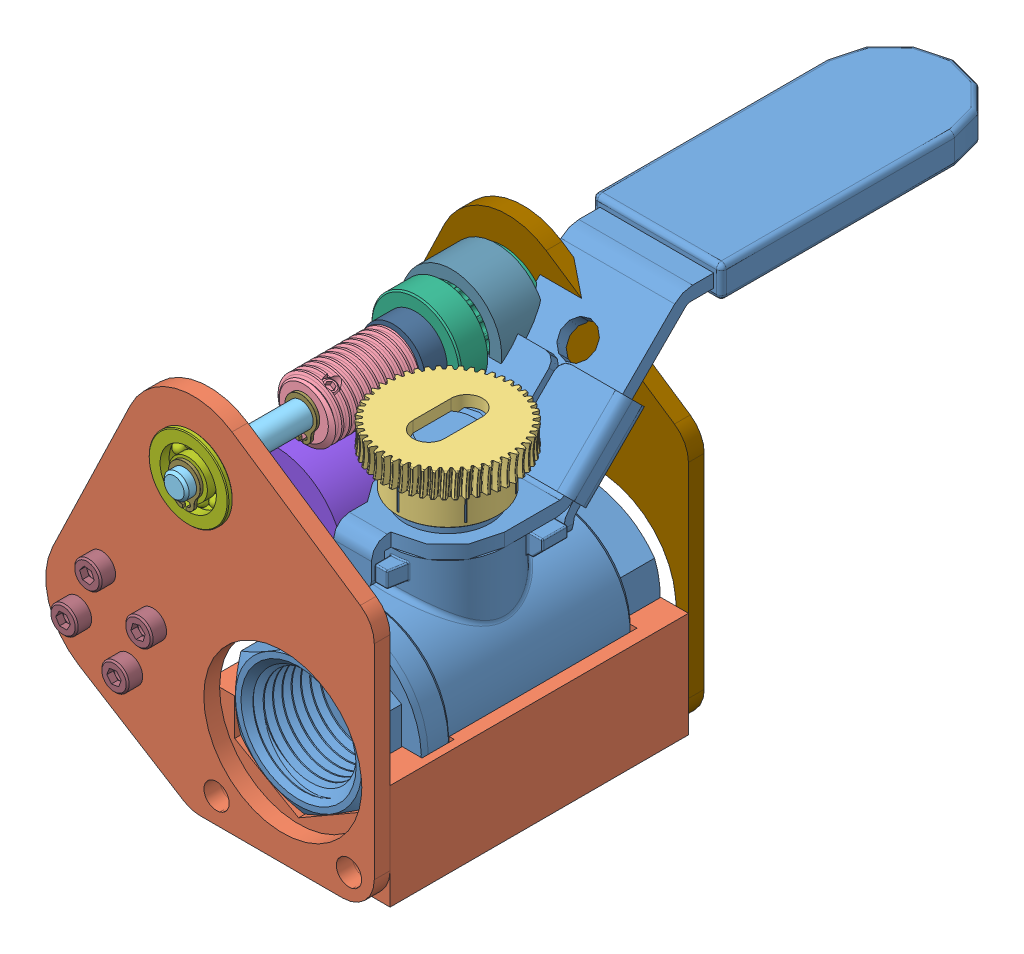
SolidWorks assembly Motor Actuated Ball Valve, configuration Default. Lengths in mm.
Overall size (75.06 72.35 73.93).
21 component instances, 14 part files, 42 mates.
Components (placement in the parent):
- 46495K21_Ultra-Corrosion Resistant Full-Port On-Off Valve-1: 46495K21_Ultra-Corrosion Resistant Full-Port On-Off Valve [46495K21] at origin size (33.34 68.26 131.76)
- Valve Actuator Mount-1: Valve Actuator Mount [Default] at (0 0.0196 29.972) size (66 72.35 63.12)
- 57545K739_Metal Worm Gear(1)-1: 57545K739_Metal Worm Gear(1) [57545K739] at (0 37.2178 0) x (1 0 0) z (0 1 0) size (26.45 26.47 12.01)
- 57545K624_Steel Worm(2)-1: 57545K624_Steel Worm(2) [57545K624] at (-18 37.2178 1.922) x (0.87687 -0.480728 0) z (0 0 1) size (12.31 12.28 18.47)
- 1327K51_Rotary Shaft-1: 1327K51_Rotary Shaft [1327K51] at (-18 37.2178 -0.5366) x (-0.408826 -0.912612 0) z (0 0 1) size (5 5 73.93)
- 3764N124_High-Strength Gt Timing Belt Pulley(1)-1: 3764N124_High-Strength Gt Timing Belt Pulley(1) [3764N124] at (-18 37.2178 -20.298) x (-0.904073 -0.427377 0) z (0 0 1) size (18.03 18.03 17.55)
- 57155K466_Flanged Ball Bearing-1: 57155K466_Flanged Ball Bearing [57155K466] at (-18 37.2178 31.647) x (-0.923728 -0.383049 0) z (0 0 -1) size (16 16 5)
- 1950KV Motor Simplified-1: 1950KV Motor Simplified [Default] at (-33.6232 4.7845 7.127) x (0.905404 -0.424552 0) z (0.424552 0.905404 0) size (27.9 30.65 27.9)
- MainPlate-1: MainPlate [Default] at (0 0.0196 -33.147) size (66 72.35 3.17)
- 57155K466_Flanged Ball Bearing-2: 57155K466_Flanged Ball Bearing [57155K466] at (-18 37.2178 -31.647) x (1 -0.000155 0) z (0 0 1) size (16 16 5)
- 3764N124_High-Strength Gt Timing Belt Pulley(1)-3: 3764N124_High-Strength Gt Timing Belt Pulley(1) [3764N124] at (-33.6232 4.7845 -20.298) x (0.998535 0.054107 0) z (0 0 1) size (18.03 18.03 17.55)
- Spacer-1: Spacer [Default] at (-18 37.2178 -11.523) x (-0.217642 -0.976029 0) z (-0.976029 0.217642 0) size (12.7 4.45 12.7)
- Part5^Motor Actuated Ball Valve-1: Part5^Motor Actuated Ball Valve [Default] at (-33.6232 4.7845 7.127) x (-0.905404 0.424552 0) z (0 0 1) size (22.86 22.86 22.85) (virtual)
- 98541A113_External Retaining Ring-1: 98541A113_External Retaining Ring [98541A113] at (-18 36.5177 34.647) size (6.43 8.3 0.6)
- 98541A113_External Retaining Ring-2: 98541A113_External Retaining Ring [98541A113] at (-18 36.5177 -34.647) size (6.43 8.3 0.6)
- 98541A113_External Retaining Ring-3: 98541A113_External Retaining Ring [98541A113] at (-18 36.5177 11.222) size (6.43 8.3 0.6)
- socket head cap screw_am-20: socket head cap screw_am [B18.3.1M - 3 x 0.5 x 30 Hex SHCS -- 18NHX] at (-36.3434 12.3079 36.147) x (0 0 -1) z (-0.923728 -0.383049 0) size (33 5.5 5.5)
- socket head cap screw_am-21: socket head cap screw_am [B18.3.1M - 3 x 0.5 x 30 Hex SHCS -- 18NHX] at (-41.1466 2.0644 36.147) x (0 0 -1) z (-0.85131 -0.524663 0) size (33 5.5 5.5)
- socket head cap screw_am-23: socket head cap screw_am [B18.3.1M - 3 x 0.5 x 30 Hex SHCS -- 18NHX] at (-30.9031 -2.7388 36.147) x (0 0 -1) z (-0.777574 -0.628792 0) size (33 5.5 5.5)
- socket head cap screw_am-25: socket head cap screw_am [B18.3.1M - 3 x 0.5 x 30 Hex SHCS -- 18NHX] at (-26.0999 7.5046 36.147) x (0 0 -1) z (-0.715577 -0.698533 0) size (33 5.5 5.5)
- Part7^Motor Actuated Ball Valve-1: Part7^Motor Actuated Ball Valve [Default] at (-18 37.2178 -27.803) x (-0.904073 -0.427377 0) z (0 0 1) size (48.08 42.73 9) (virtual)
Mates (geometry in assembly coordinates):
- Width1: width anti-aligned: plane of Valve Actuator Mount-1 through (-12.827 0.0196 21.9794) normal (1 0 0); plane of 46495K21_Ultra-Corrosion Resistant Full-Port On-Off Valve-1 through (12.827 0.0196 21.9794) normal (-1 0 0); plane of Valve Actuator Mount-1 through (-12.7 7.3323 29.972) normal (-1 0 0); plane of 46495K21_Ultra-Corrosion Resistant Full-Port On-Off Valve-1 through (12.7 -7.3323 29.972) normal (1 0 0)
- Distance1: distance = 0.127 mm: line of Valve Actuator Mount-1 through (0 -14.7917 21.9794) axis (0 0 1); line of 46495K21_Ultra-Corrosion Resistant Full-Port On-Off Valve-1 through (0 -14.6647 28.8377) axis (0 0 -1)
- Coincident2: coincident aligned: plane of 46495K21_Ultra-Corrosion Resistant Full-Port On-Off Valve-1 through (0 0 29.972) normal (0 0 1); plane of Valve Actuator Mount-1 through (0 0.0196 29.972) normal (0 0 1)
- Concentric1: concentric anti-aligned: circle of 46495K21_Ultra-Corrosion Resistant Full-Port On-Off Valve-1; circle of 57545K739_Metal Worm Gear(1)-1
- Coincident3: coincident anti-aligned: plane of 46495K21_Ultra-Corrosion Resistant Full-Port On-Off Valve-1 through (0 27.7177 0) normal (0 1 0); plane of 57545K739_Metal Worm Gear(1)-1 through (0 27.7177 0) normal (0 -1 0)
- Concentric2: concentric aligned: cylinder of 57545K624_Steel Worm(2)-1 through (-18 37.2178 -7.078) axis (0 0 -1) radius 2.5; cylinder of 1327K51_Rotary Shaft-1 through (-18 37.2178 49.4634) axis (0 0 -1) radius 2.5
- Concentric3: concentric aligned: cylinder of Valve Actuator Mount-1 through (-18 37.2178 33.147) axis (0 0 -1) radius 7; cylinder of 57155K466_Flanged Ball Bearing-1 through (-18 37.2178 31.647) axis (0 0 -1) radius 7
- Coincident4: coincident anti-aligned: plane of Valve Actuator Mount-1 through (-18 37.2178 33.147) normal (0 0 1); plane of 57155K466_Flanged Ball Bearing-1 through (-21.0644 44.6076 33.147) normal (0 0 -1)
- Concentric4: concentric aligned: cylinder of 1327K51_Rotary Shaft-1 through (-18 37.2178 49.4634) axis (0 0 -1) radius 2.5; cylinder of 57155K466_Flanged Ball Bearing-1 through (-18 37.2178 31.647) axis (0 0 -1) radius 2.5
- Distance2: distance = 19.05 mm anti-aligned: plane of 57545K624_Steel Worm(2)-1 through (-18 37.2178 10.922) normal (0 0 1); plane of Valve Actuator Mount-1 through (-18 37.2178 29.972) normal (0 0 -1)
- Concentric7: concentric anti-aligned: cylinder of Valve Actuator Mount-1 through (-41.1466 2.0644 29.972) axis (0 0 -1) radius 1.45; cylinder of 1950KV Motor Simplified-1 through (-41.1466 2.0644 7.127) axis (0 0 1) radius 1.45
- Concentric8: concentric anti-aligned: cylinder of Valve Actuator Mount-1 through (-36.3434 12.3079 29.972) axis (0 0 -1) radius 1.45; cylinder of 1950KV Motor Simplified-1 through (-36.3434 12.3079 7.127) axis (0 0 1) radius 1.45
- Concentric9: concentric aligned: cylinder of Valve Actuator Mount-1 through (13.3033 -16.0617 33.147) axis (0 0 -1) radius 2.54; cylinder of MainPlate-1 through (13.3033 -16.0617 -29.972) axis (0 0 -1) radius 2.54
- Coincident7: coincident anti-aligned: plane of Valve Actuator Mount-1 through (0 0.0196 -29.972) normal (0 0 -1); plane of MainPlate-1 through (-18 37.2178 -29.972) normal (0 0 1)
- Concentric10: concentric aligned: cylinder of Valve Actuator Mount-1 through (-13.3033 -16.0617 33.147) axis (0 0 -1) radius 2.54; cylinder of MainPlate-1 through (-13.3033 -16.0617 -29.972) axis (0 0 -1) radius 2.54
- Concentric11: concentric aligned: circle of MainPlate-1; circle of 57155K466_Flanged Ball Bearing-2
- Coincident8: coincident anti-aligned: plane of MainPlate-1 through (-18 37.2178 -33.147) normal (0 0 -1); plane of 57155K466_Flanged Ball Bearing-2 through (-17.9988 45.2177 -33.147) normal (0 0 1)
- Coincident9: coincident anti-aligned: plane of 1950KV Motor Simplified-1 through (-33.6232 4.7845 -11.523) normal (0 0 -1); plane of 3764N124_High-Strength Gt Timing Belt Pulley(1)-3 through (-33.4944 2.4068 -11.523) normal (0 0 1)
- Concentric15: concentric anti-aligned: cylinder of 1950KV Motor Simplified-1 through (-33.6232 4.7845 7.127) axis (0 0 1) radius 2.5; cylinder of 3764N124_High-Strength Gt Timing Belt Pulley(1)-3 through (-33.6232 4.7845 -11.523) axis (0 0 -1) radius 2.5
- Concentric16: concentric aligned: cylinder of 1327K51_Rotary Shaft-1 through (-18 37.2178 49.4634) axis (0 0 -1) radius 2.5; cylinder of 3764N124_High-Strength Gt Timing Belt Pulley(1)-1 through (-18 37.2178 -11.523) axis (0 0 -1) radius 2.5
- Coincident10: coincident aligned: plane of 3764N124_High-Strength Gt Timing Belt Pulley(1)-1 through (-21.8528 45.368 -29.073) normal (0 0 -1); plane of 3764N124_High-Strength Gt Timing Belt Pulley(1)-3 through (-33.1355 -4.2173 -29.073) normal (0 0 -1)
- ProfileCenter1: profile center aligned: circle of Spacer-1; circle of 57545K624_Steel Worm(2)-1
- Coincident11: coincident anti-aligned: plane of 3764N124_High-Strength Gt Timing Belt Pulley(1)-1 through (-19.0177 39.3706 -11.523) normal (0 0 1); plane of Spacer-1 through (-18 37.2178 -11.523) normal (0 0 -1)
- InPlace1: in place: plane of ? through (-33.6232 7.0198 7.127) normal (0 0 1); plane of ? through (0 0 7.127) normal (0 0 1); moOrthogonalPlaneRef_w of ? through (-33.6232 7.0198 7.127) normal (0 0 1); plane of ? through (0 0 7.127) normal (0 1 0); plane of ? through (-33.6232 7.0198 7.127) normal (0 0 1); plane of ? through (0 0 7.127) normal (1 0 0); plane of 1950KV Motor Simplified-1 through (-33.6232 4.7845 7.127) normal (0 0 1); unknown of Part5^Motor Actuated Ball Valve-1
- Coincident12: coincident aligned: plane of 1950KV Motor Simplified-1; plane of Part5^Motor Actuated Ball Valve-1
- Coincident13: coincident aligned: moOrthogonalPlaneRef_w of 1950KV Motor Simplified-1 through (-33.6232 4.7845 7.127) normal (-0.424552 -0.905404 0); plane of Part5^Motor Actuated Ball Valve-1 through (-33.6232 4.7845 7.127) normal (-0.424552 -0.905404 0)
- Coincident14: coincident anti-aligned: moOrthogonalPlaneRef_w of 1950KV Motor Simplified-1 through (-33.6232 4.7845 7.127) normal (0.905404 -0.424552 0); plane of Part5^Motor Actuated Ball Valve-1 through (-33.6232 4.7845 7.127) normal (-0.905404 0.424552 0)
- Concentric20: concentric anti-aligned: circle of 1327K51_Rotary Shaft-1; circle of 98541A113_External Retaining Ring-1
- Coincident15: coincident anti-aligned: plane of 1327K51_Rotary Shaft-1 through (-18.9812 35.0275 34.347) normal (0 0 1); plane of 98541A113_External Retaining Ring-1 through (-21.9381 34.1292 34.347) normal (0 0 -1)
- Concentric21: concentric aligned: cylinder of 1327K51_Rotary Shaft-1 through (-18 37.2178 49.4634) axis (0 0 -1) radius 2.5; cylinder of 98541A113_External Retaining Ring-3 through (-18 37.2178 11.522) axis (0 0 -1) radius 2.35
- Coincident16: coincident anti-aligned: plane of 1327K51_Rotary Shaft-1 through (-18.9812 35.0275 10.922) normal (0 0 1); plane of 98541A113_External Retaining Ring-3 through (-21.9381 34.1292 10.922) normal (0 0 -1)
- Concentric22: concentric anti-aligned: cylinder of 1327K51_Rotary Shaft-1 through (-18 37.2178 49.4634) axis (0 0 1) radius 2.4; cylinder of 98541A113_External Retaining Ring-2 through (-18 37.2178 -34.347) axis (0 0 -1) radius 2.35
- Coincident17: coincident aligned: plane of 1327K51_Rotary Shaft-1 through (-18.9812 35.0275 -34.347) normal (0 0 -1); circle of 98541A113_External Retaining Ring-2
- Coincident18: coincident anti-aligned: plane of 57545K624_Steel Worm(2)-1 through (-18 37.2178 10.922) normal (0 0 1); plane of 98541A113_External Retaining Ring-3 through (-21.9381 34.1292 10.922) normal (0 0 -1)
- ProfileCenter2: profile center anti-aligned: circle of socket head cap screw_am-20; circle of Valve Actuator Mount-1
- ProfileCenter3: profile center anti-aligned: circle of socket head cap screw_am-21; circle of Valve Actuator Mount-1
- ProfileCenter4: profile center anti-aligned: circle of socket head cap screw_am-23; circle of Valve Actuator Mount-1
- ProfileCenter5: profile center anti-aligned: circle of socket head cap screw_am-25; circle of Valve Actuator Mount-1
- InPlace2: in place: plane of 3764N124_High-Strength Gt Timing Belt Pulley(1)-1 through (-21.1047 43.7854 -27.803) normal (0 0 1); plane of ? through (0 0 -27.803) normal (0 0 1); plane of 3764N124_High-Strength Gt Timing Belt Pulley(1)-1 through (-21.1047 43.7854 -27.803) normal (0 0 1); plane of ? through (0 0 -27.803) normal (0 1 0); plane of 3764N124_High-Strength Gt Timing Belt Pulley(1)-1 through (-21.1047 43.7854 -27.803) normal (0 0 1); plane of ? through (0 0 -27.803) normal (1 0 0); plane of 3764N124_High-Strength Gt Timing Belt Pulley(1)-1 through (-21.1047 43.7854 -27.803) normal (0 0 1); unknown of Part7^Motor Actuated Ball Valve-1
- Coincident19: coincident aligned: plane of 3764N124_High-Strength Gt Timing Belt Pulley(1)-1; plane of Part7^Motor Actuated Ball Valve-1
- Coincident20: coincident aligned: moOrthogonalPlaneRef_w of 3764N124_High-Strength Gt Timing Belt Pulley(1)-1 through (-18 37.2178 -27.803) normal (0.427377 -0.904073 0); plane of Part7^Motor Actuated Ball Valve-1 through (-18 37.2178 -27.803) normal (0.427377 -0.904073 0)
- Coincident21: coincident anti-aligned: moOrthogonalPlaneRef_w of 3764N124_High-Strength Gt Timing Belt Pulley(1)-1 through (-18 37.2178 -27.803) normal (0.904073 0.427377 0); plane of Part7^Motor Actuated Ball Valve-1 through (-18 37.2178 -27.803) normal (-0.904073 -0.427377 0)
